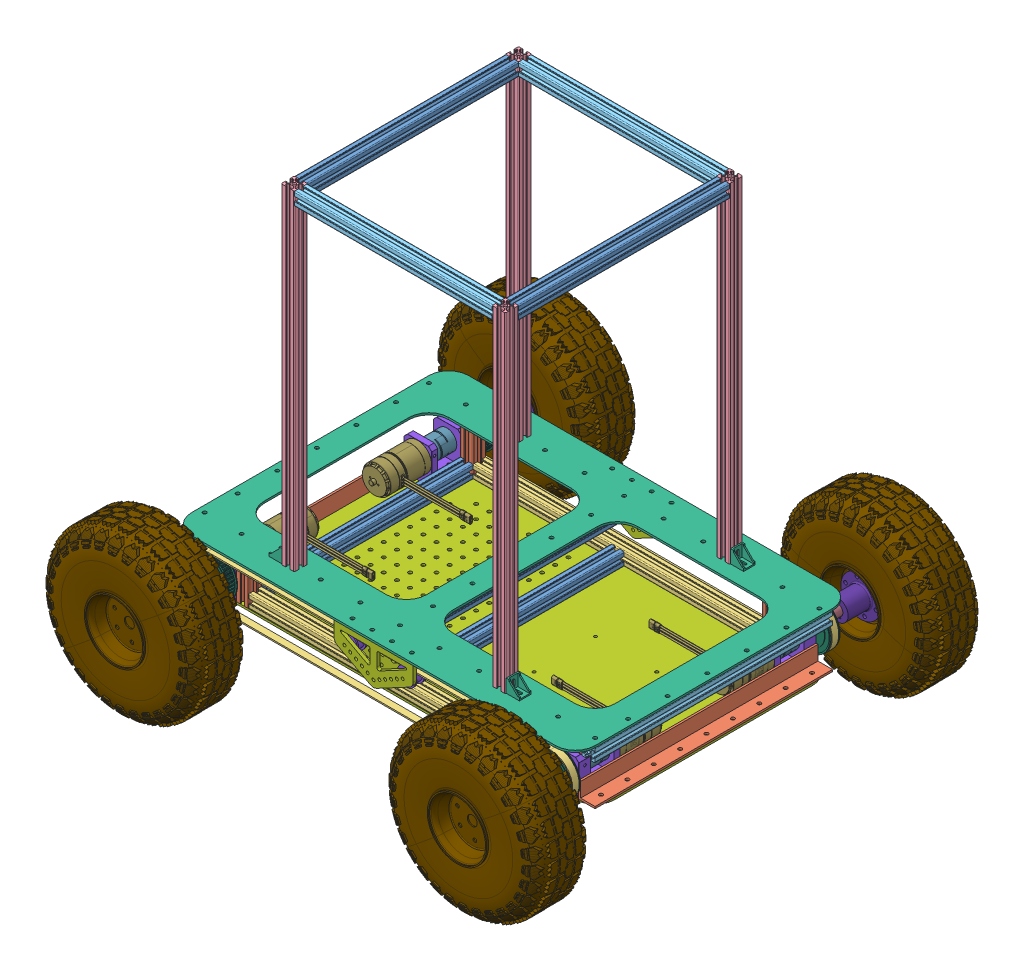
SolidWorks assembly 总装, configuration 默认. Lengths in mm.
Overall size (861.9 722.49 686.75).
130 component instances, 27 part files, 43 mates.
Components (placement in the parent):
- 框架-1: 框架 [默认] at (-91.5436 0.0792 612) size (612 80 360) (flexible)
  - 320-1: 320 [默认] at (-239 0 -160) size (20 20 320)
  - 60-1: 60 [默认] at (-239 0 160) x (0 0 1) z (0 1 0) size (20 20 60)
  - 60-2: 60 [默认] at (-239 60 -180) x (1 0 0) z (0 -1 0) size (20 20 60)
  - 438-1: 438 [默认] at (-219 0 180) x (0 0 -1) z (1 0 0) size (20 20 438)
  - 438-2: 438 [默认] at (-219 0 -160) x (0 0 -1) z (1 0 0) size (20 20 438)
  - 60-3: 60 [默认] at (219 60 -180) x (1 0 0) z (0 -1 0) size (20 20 60)
  - 60-4: 60 [默认] at (219 60 160) x (1 0 0) z (0 -1 0) size (20 20 60)
  - 320-2: 320 [默认] at (219 0 -160) size (20 20 320)
  - 572-3: 572 [默认] at (-286 60 180) x (0 0 -1) z (1 0 0) size (20 20 572)
  - 572-4: 572 [默认] at (-286 60 -160) x (0 0 -1) z (1 0 0) size (20 20 572)
  - 360-3: 360 [默认] at (-306 60 -180) size (20 20 360)
  - 360-4: 360 [默认] at (286 60 -180) size (20 20 360)
  - 320-3: 320 [默认] at (-10 60 -160) size (20 20 320)
  - 320-4: 320 [默认] at (-10 0 -160) size (20 20 320)
- 铝底板-上-1: 铝底板-上 [默认] at (-91.5436 80.0792 612) x (0 0 -1) z (1 0 0) size (420 3 612)
- 铝底板-下-1: 铝底板-下 [默认] at (-91.5436 -2.9208 612) x (0 0 1) z (-1 0 0) size (360 3 612)
- 轮胎模组-1: 轮胎模组 [默认] at (230.9564 22.3703 451.1678) x (0 0 -1) z (-1 0 0) size (297.23 295.63 295.43) (flexible)
  - m3508-1: m3508 [Default] at (-12.228 0.9134 62.5) size (62.5 52.5 42)
  - deep groove ball bearings gb-1: deep groove ball bearings gb [Rolling bearings 6000 GB 276-94] at (6.9178 -9.2089 62.5) size (8 26 26)
  - deep groove ball bearings gb-2: deep groove ball bearings gb [Rolling bearings 6000 GB 276-94] at (14.9178 -9.2089 62.5) x (1 0 0) z (0 0.136617 0.990624) size (8 26 26)
  - plain washers for clevis pins gb-1: plain washers for clevis pins gb [GB_ROUND_WASHERS_TYPE7 3] at (19.7178 1.5391 73.248) x (0 0 -1) z (1 0 0) size (6 6 0.8)
  - plain washers for clevis pins gb-2: plain washers for clevis pins gb [GB_ROUND_WASHERS_TYPE7 3] at (19.7178 1.5391 51.752) x (0 0 -1) z (1 0 0) size (6 6 0.8)
  - plain washers for clevis pins gb-3: plain washers for clevis pins gb [GB_ROUND_WASHERS_TYPE7 3] at (19.7178 -20.4006 72.7853) x (0 0 -1) z (1 0 0) size (6 6 0.8)
  - plain washers for clevis pins gb-4: plain washers for clevis pins gb [GB_ROUND_WASHERS_TYPE7 3] at (19.7178 -19.4942 51.3083) x (0 0 -1) z (1 0 0) size (6 6 0.8)
  - hexagon socket head cap screws gb-1: hexagon socket head cap screws gb [GB_FASTENER_SCREWS_HSHCS M3X8-N] at (22.7178 1.5391 73.248) x (-1 0 0) z (0 0.924225 0.381849) size (11 5.5 5.5)
  - hexagon socket head cap screws gb-2: hexagon socket head cap screws gb [GB_FASTENER_SCREWS_HSHCS M3X8-N] at (22.7178 1.5391 51.752) x (-1 0 0) z (0 0.924225 0.381849) size (11 5.5 5.5)
  - hexagon socket head cap screws gb-3: hexagon socket head cap screws gb [GB_FASTENER_SCREWS_HSHCS M3X8-N] at (22.7178 -20.4006 72.7853) x (-1 0 0) z (0 0.924225 0.381849) size (11 5.5 5.5)
  - hexagon socket head cap screws gb-4: hexagon socket head cap screws gb [GB_FASTENER_SCREWS_HSHCS M3X8-N] at (22.7178 -19.4942 51.3083) x (-1 0 0) z (0 0.924225 0.381849) size (11 5.5 5.5)
  - RoboMaster M3508直流无刷减速电-1: RoboMaster M3508直流无刷减速电 [默认] at (-130.0232 -5.4389 80.4643) x (0 -0.954008 0.299781) z (1 0 0) size (63.71 141.17 98.4)
  - 轴-1: 轴 [默认] at (18.9178 -9.2089 62.5) x (0 0.969975 -0.243205) z (0 0.243205 0.969975) size (16 128 16)
  - CPJCK30-RD-10-10-1: CPJCK30-RD-10-10 [Default] at (-34.3322 -9.2089 62.5) x (1 0 0) z (0 0.124503 0.992219) size (35 30 30)
  - 同步轮-1: 同步轮 [Default] at (28.0178 -9.2089 62.5) x (1 0 0) z (0 0.430878 0.90241) size (16 67 67)
  - 平键5x5x35-1: 平键5x5x35 [默认] at (94.4178 -1.9341 60.676) x (0 0.243205 0.969975) z (0 -0.969975 0.243205) size (5 41 5)
  - 法兰-1: 法兰 [默认] at (113.9178 -9.2089 62.5) x (0 -0.243205 -0.969975) z (1 0 0) size (60 60 41)
  - 10寸充气轮-1: 10寸充气轮 [Default] at (181.1138 -156.8863 150.0145) x (0 0.247823 -0.968805) z (1 0 0) size (242.76 243.05 91.75)
  - circlips for shaft--type a large gb-1: circlips for shaft--type a large gb [GB_CONNECTING_PIECE_RING_RRA 16] at (28.0178 -8.6289 62.5) x (0 0 -1) z (1 0 0) size (18.2 20.68 1)
  - circlips for shaft--type a large gb-2: circlips for shaft--type a large gb [GB_CONNECTING_PIECE_RING_RRA 16] at (44.0178 -8.6289 62.5) x (0 0 1) z (-1 0 0) size (18.2 20.68 1)
- 轮胎模组-2: 轮胎模组 [默认] at (105.9564 22.3703 772.8322) x (0 0 1) z (1 0 0) size (297.23 341.76 341.72) (flexible)
  - m3508-1: m3508 [Default] at (-12.228 0.9134 62.5) size (62.5 52.5 42)
  - deep groove ball bearings gb-1: deep groove ball bearings gb [Rolling bearings 6000 GB 276-94] at (6.9178 -9.2089 62.5) size (8 26 26)
  - deep groove ball bearings gb-2: deep groove ball bearings gb [Rolling bearings 6000 GB 276-94] at (14.9178 -9.2089 62.5) x (1 0 0) z (0 0.136617 0.990624) size (8 26 26)
  - plain washers for clevis pins gb-1: plain washers for clevis pins gb [GB_ROUND_WASHERS_TYPE7 3] at (19.7178 1.5391 73.248) x (0 0 -1) z (1 0 0) size (6 6 0.8)
  - plain washers for clevis pins gb-2: plain washers for clevis pins gb [GB_ROUND_WASHERS_TYPE7 3] at (19.7178 1.5391 51.752) x (0 0 -1) z (1 0 0) size (6 6 0.8)
  - plain washers for clevis pins gb-3: plain washers for clevis pins gb [GB_ROUND_WASHERS_TYPE7 3] at (19.7178 -20.4006 72.7853) x (0 0 -1) z (1 0 0) size (6 6 0.8)
  - plain washers for clevis pins gb-4: plain washers for clevis pins gb [GB_ROUND_WASHERS_TYPE7 3] at (19.7178 -19.4942 51.3083) x (0 0 -1) z (1 0 0) size (6 6 0.8)
  - hexagon socket head cap screws gb-1: hexagon socket head cap screws gb [GB_FASTENER_SCREWS_HSHCS M3X8-N] at (22.7178 1.5391 73.248) x (-1 0 0) z (0 0.924225 0.381849) size (11 5.5 5.5)
  - hexagon socket head cap screws gb-2: hexagon socket head cap screws gb [GB_FASTENER_SCREWS_HSHCS M3X8-N] at (22.7178 1.5391 51.752) x (-1 0 0) z (0 0.924225 0.381849) size (11 5.5 5.5)
  - hexagon socket head cap screws gb-3: hexagon socket head cap screws gb [GB_FASTENER_SCREWS_HSHCS M3X8-N] at (22.7178 -20.4006 72.7853) x (-1 0 0) z (0 0.924225 0.381849) size (11 5.5 5.5)
  - hexagon socket head cap screws gb-4: hexagon socket head cap screws gb [GB_FASTENER_SCREWS_HSHCS M3X8-N] at (22.7178 -19.4942 51.3083) x (-1 0 0) z (0 0.924225 0.381849) size (11 5.5 5.5)
  - RoboMaster M3508直流无刷减速电-1: RoboMaster M3508直流无刷减速电 [默认] at (-130.0232 -12.9789 44.5357) x (0 0.954008 -0.299781) z (1 0 0) size (63.71 141.17 98.4)
  - 轴-1: 轴 [默认] at (18.9178 -9.2089 62.5) x (0 0.982488 0.186325) z (0 -0.186325 0.982488) size (16 128 16)
  - CPJCK30-RD-10-10-1: CPJCK30-RD-10-10 [Default] at (-34.3322 -9.2089 62.5) x (1 0 0) z (0 0.124503 0.992219) size (35 30 30)
  - 同步轮-1: 同步轮 [Default] at (28.0178 -9.2089 62.5) size (16 67 67)
  - 平键5x5x35-1: 平键5x5x35 [默认] at (94.4178 -1.8402 63.8974) x (0 -0.186325 0.982488) z (0 -0.982488 -0.186325) size (5 41 5)
  - 法兰-1: 法兰 [默认] at (113.9178 -9.2089 62.5) x (0 0.186325 -0.982488) z (1 0 0) size (60 60 41)
  - 10寸充气轮-1: 10寸充气轮 [Default] at (181.1138 -179.9795 79.9579) x (0 0.631528 -0.775353) z (1 0 0) size (242.76 243.05 91.75)
  - circlips for shaft--type a large gb-1: circlips for shaft--type a large gb [GB_CONNECTING_PIECE_RING_RRA 16] at (28.0178 -8.6289 62.5) x (0 0 -1) z (1 0 0) size (18.2 20.68 1)
  - circlips for shaft--type a large gb-2: circlips for shaft--type a large gb [GB_CONNECTING_PIECE_RING_RRA 16] at (44.0178 -8.6289 62.5) x (0 0 1) z (-1 0 0) size (18.2 20.68 1)
- 轮胎模组-5: 轮胎模组 [默认] at (-289.0436 22.3703 451.1678) x (0 0 -1) z (-1 0 0) size (297.23 341.76 341.72) (flexible)
  - m3508-1: m3508 [Default] at (-12.228 0.9134 62.5) size (62.5 52.5 42)
  - deep groove ball bearings gb-1: deep groove ball bearings gb [Rolling bearings 6000 GB 276-94] at (6.9178 -9.2089 62.5) size (8 26 26)
  - deep groove ball bearings gb-2: deep groove ball bearings gb [Rolling bearings 6000 GB 276-94] at (14.9178 -9.2089 62.5) x (1 0 0) z (0 0.136617 0.990624) size (8 26 26)
  - plain washers for clevis pins gb-1: plain washers for clevis pins gb [GB_ROUND_WASHERS_TYPE7 3] at (19.7178 1.5391 73.248) x (0 0 -1) z (1 0 0) size (6 6 0.8)
  - plain washers for clevis pins gb-2: plain washers for clevis pins gb [GB_ROUND_WASHERS_TYPE7 3] at (19.7178 1.5391 51.752) x (0 0 -1) z (1 0 0) size (6 6 0.8)
  - plain washers for clevis pins gb-3: plain washers for clevis pins gb [GB_ROUND_WASHERS_TYPE7 3] at (19.7178 -20.4006 72.7853) x (0 0 -1) z (1 0 0) size (6 6 0.8)
  - plain washers for clevis pins gb-4: plain washers for clevis pins gb [GB_ROUND_WASHERS_TYPE7 3] at (19.7178 -19.4942 51.3083) x (0 0 -1) z (1 0 0) size (6 6 0.8)
  - hexagon socket head cap screws gb-1: hexagon socket head cap screws gb [GB_FASTENER_SCREWS_HSHCS M3X8-N] at (22.7178 1.5391 73.248) x (-1 0 0) z (0 0.924225 0.381849) size (11 5.5 5.5)
  - hexagon socket head cap screws gb-2: hexagon socket head cap screws gb [GB_FASTENER_SCREWS_HSHCS M3X8-N] at (22.7178 1.5391 51.752) x (-1 0 0) z (0 0.924225 0.381849) size (11 5.5 5.5)
  - hexagon socket head cap screws gb-3: hexagon socket head cap screws gb [GB_FASTENER_SCREWS_HSHCS M3X8-N] at (22.7178 -20.4006 72.7853) x (-1 0 0) z (0 0.924225 0.381849) size (11 5.5 5.5)
  - hexagon socket head cap screws gb-4: hexagon socket head cap screws gb [GB_FASTENER_SCREWS_HSHCS M3X8-N] at (22.7178 -19.4942 51.3083) x (-1 0 0) z (0 0.924225 0.381849) size (11 5.5 5.5)
  - RoboMaster M3508直流无刷减速电-1: RoboMaster M3508直流无刷减速电 [默认] at (-130.0232 -12.9789 44.5357) x (0 0.954008 -0.299781) z (1 0 0) size (63.71 141.17 98.4)
  - 轴-1: 轴 [默认] at (18.9178 -9.2089 62.5) x (0 0.982488 0.186325) z (0 -0.186325 0.982488) size (16 128 16)
  - CPJCK30-RD-10-10-1: CPJCK30-RD-10-10 [Default] at (-34.3322 -9.2089 62.5) x (1 0 0) z (0 0.124503 0.992219) size (35 30 30)
  - 同步轮-1: 同步轮 [Default] at (28.0178 -9.2089 62.5) size (16 67 67)
  - 平键5x5x35-1: 平键5x5x35 [默认] at (94.4178 -1.8402 63.8974) x (0 -0.186325 0.982488) z (0 -0.982488 -0.186325) size (5 41 5)
  - 法兰-1: 法兰 [默认] at (113.9178 -9.2089 62.5) x (0 0.186325 -0.982488) z (1 0 0) size (60 60 41)
  - 10寸充气轮-1: 10寸充气轮 [Default] at (181.1138 -179.9795 79.9579) x (0 0.631528 -0.775353) z (1 0 0) size (242.76 243.05 91.75)
  - circlips for shaft--type a large gb-1: circlips for shaft--type a large gb [GB_CONNECTING_PIECE_RING_RRA 16] at (28.0178 -8.6289 62.5) x (0 0 -1) z (1 0 0) size (18.2 20.68 1)
  - circlips for shaft--type a large gb-2: circlips for shaft--type a large gb [GB_CONNECTING_PIECE_RING_RRA 16] at (44.0178 -8.6289 62.5) x (0 0 1) z (-1 0 0) size (18.2 20.68 1)
- 轮胎模组-6: 轮胎模组 [默认] at (-414.0436 22.3703 772.8322) x (0 0 1) z (1 0 0) size (297.23 341.76 341.72) (flexible)
  - m3508-1: m3508 [Default] at (-12.228 0.9134 62.5) size (62.5 52.5 42)
  - deep groove ball bearings gb-1: deep groove ball bearings gb [Rolling bearings 6000 GB 276-94] at (6.9178 -9.2089 62.5) size (8 26 26)
  - deep groove ball bearings gb-2: deep groove ball bearings gb [Rolling bearings 6000 GB 276-94] at (14.9178 -9.2089 62.5) x (1 0 0) z (0 0.136617 0.990624) size (8 26 26)
  - plain washers for clevis pins gb-1: plain washers for clevis pins gb [GB_ROUND_WASHERS_TYPE7 3] at (19.7178 1.5391 73.248) x (0 0 -1) z (1 0 0) size (6 6 0.8)
  - plain washers for clevis pins gb-2: plain washers for clevis pins gb [GB_ROUND_WASHERS_TYPE7 3] at (19.7178 1.5391 51.752) x (0 0 -1) z (1 0 0) size (6 6 0.8)
  - plain washers for clevis pins gb-3: plain washers for clevis pins gb [GB_ROUND_WASHERS_TYPE7 3] at (19.7178 -20.4006 72.7853) x (0 0 -1) z (1 0 0) size (6 6 0.8)
  - plain washers for clevis pins gb-4: plain washers for clevis pins gb [GB_ROUND_WASHERS_TYPE7 3] at (19.7178 -19.4942 51.3083) x (0 0 -1) z (1 0 0) size (6 6 0.8)
  - hexagon socket head cap screws gb-1: hexagon socket head cap screws gb [GB_FASTENER_SCREWS_HSHCS M3X8-N] at (22.7178 1.5391 73.248) x (-1 0 0) z (0 0.924225 0.381849) size (11 5.5 5.5)
  - hexagon socket head cap screws gb-2: hexagon socket head cap screws gb [GB_FASTENER_SCREWS_HSHCS M3X8-N] at (22.7178 1.5391 51.752) x (-1 0 0) z (0 0.924225 0.381849) size (11 5.5 5.5)
  - hexagon socket head cap screws gb-3: hexagon socket head cap screws gb [GB_FASTENER_SCREWS_HSHCS M3X8-N] at (22.7178 -20.4006 72.7853) x (-1 0 0) z (0 0.924225 0.381849) size (11 5.5 5.5)
  - hexagon socket head cap screws gb-4: hexagon socket head cap screws gb [GB_FASTENER_SCREWS_HSHCS M3X8-N] at (22.7178 -19.4942 51.3083) x (-1 0 0) z (0 0.924225 0.381849) size (11 5.5 5.5)
  - RoboMaster M3508直流无刷减速电-1: RoboMaster M3508直流无刷减速电 [默认] at (-130.0232 -5.4389 80.4643) x (0 -0.954008 0.299781) z (1 0 0) size (63.71 141.17 98.4)
  - 轴-1: 轴 [默认] at (18.9178 -9.2089 62.5) x (0 0.982488 0.186325) z (0 -0.186325 0.982488) size (16 128 16)
  - CPJCK30-RD-10-10-1: CPJCK30-RD-10-10 [Default] at (-34.3322 -9.2089 62.5) x (1 0 0) z (0 0.124503 0.992219) size (35 30 30)
  - 同步轮-1: 同步轮 [Default] at (28.0178 -9.2089 62.5) size (16 67 67)
  - 平键5x5x35-1: 平键5x5x35 [默认] at (94.4178 -1.8402 63.8974) x (0 -0.186325 0.982488) z (0 -0.982488 -0.186325) size (5 41 5)
  - 法兰-1: 法兰 [默认] at (113.9178 -9.2089 62.5) x (0 0.186325 -0.982488) z (1 0 0) size (60 60 41)
  - 10寸充气轮-1: 10寸充气轮 [Default] at (181.1138 -179.9795 79.9579) x (0 0.631528 -0.775353) z (1 0 0) size (242.76 243.05 91.75)
  - circlips for shaft--type a large gb-1: circlips for shaft--type a large gb [GB_CONNECTING_PIECE_RING_RRA 16] at (28.0178 -8.6289 62.5) x (0 0 -1) z (1 0 0) size (18.2 20.68 1)
  - circlips for shaft--type a large gb-2: circlips for shaft--type a large gb [GB_CONNECTING_PIECE_RING_RRA 16] at (44.0178 -8.6289 62.5) x (0 0 1) z (-1 0 0) size (18.2 20.68 1)
- 直角铝-1: 直角铝 [默认] at (-375.5436 3.0792 612) x (0 0 -1) z (1 0 0) size (360 25 25)
- 直角铝-2: 直角铝 [默认] at (192.4564 3.0792 612) x (0 0 1) z (-1 0 0) size (360 25 25)
- 同步带-1: 同步带 [默认] at (168.4564 31.5792 813.85) x (0 0 -1) z (1 0 0) size (10 67.7 587.7)
- 同步带-2: 同步带 [默认] at (168.4564 31.5792 420.15) x (0 0 -1) z (1 0 0) size (10 67.7 587.7)
- 扩展架-1: 扩展架 [默认] at (62.0081 -166.9208 766.8893) x (0 0 -1) z (0 1 0) size (360 380 500)
  - 500-1: 500 [默认] at (-25.1107 -16.4483 250) size (20 20 500)
  - 500-2: 500 [默认] at (314.8893 -16.4483 250) size (20 20 500)
  - 500-3: 500 [默认] at (314.8893 303.5517 250) size (20 20 500)
  - 500-4: 500 [默认] at (-25.1107 303.5517 250) size (20 20 500)
  - 320-1: 320 [默认] at (-5.1107 3.5517 750) x (0 -1 0) z (1 0 0) size (20 20 320)
  - 320-2: 320 [默认] at (-5.1107 323.5517 730) x (0 0 1) z (1 0 0) size (20 20 320)
  - 300-1: 300 [默认] at (-25.1107 303.5517 730) x (1 0 0) z (0 -1 0) size (20 20 300)
  - 300-2: 300 [默认] at (314.8893 303.5517 730) x (1 0 0) z (0 -1 0) size (20 20 300)
  - 角码-1: 角码 [默认] at (995.5059 87.6877 1359.6334) x (0 -1 0) z (0 0 -1) size (20 17.5 20)
  - 角码-2: 角码 [默认] at (1335.5059 87.6877 1359.6334) x (0 -1 0) z (0 0 -1) size (20 17.5 20)
  - 角码-3: 角码 [默认] at (995.5059 -1126.0817 14.136) x (0 0 -1) z (0 1 0) size (20 17.5 20)
  - 角码-4: 角码 [默认] at (-685.7273 219.4156 1359.6334) x (0 1 0) z (0 0 -1) size (20 17.5 20)
- 张紧器-1: 张紧器 [默认] at (-91.5436 80.0792 808.85) x (0 0 1) z (-1 0 0) size (30.3 58.67 120)
  - 同步轮张紧器-1: 同步轮张紧器 [默认] at origin size (30.3 58.67 120)
  - 导向轮-1: 导向轮 [默认] at (0 -25.1373 -44.1176) size (15 28 28)
  - 钢柱4x15x8-1: 钢柱4x15x8 [默认] at (0 -25.1373 -44.1176) x (0 0 1) z (0 -1 0) size (8 16 8)
  - 导向轮-2: 导向轮 [默认] at (0 -25.1373 44.1176) x (1 0 0) z (0 -0.03847 0.99926) size (15 28 28)
  - 钢柱4x15x8-2: 钢柱4x15x8 [默认] at (0 -25.1373 44.1176) x (0 0 1) z (0 -1 0) size (8 16 8)
- 张紧器-2: 张紧器 [默认] at (-91.5436 80.0792 415.15) x (0 0 -1) z (1 0 0) size (30.3 58.67 120)
  - 同步轮张紧器-1: 同步轮张紧器 [默认] at origin size (30.3 58.67 120)
  - 导向轮-1: 导向轮 [默认] at (0 -25.1373 -44.1176) size (15 28 28)
  - 钢柱4x15x8-1: 钢柱4x15x8 [默认] at (0 -25.1373 -44.1176) x (0 0 1) z (0 -1 0) size (8 16 8)
  - 导向轮-2: 导向轮 [默认] at (0 -25.1373 44.1176) x (1 0 0) z (0 -0.03847 0.99926) size (15 28 28)
  - 钢柱4x15x8-2: 钢柱4x15x8 [默认] at (0 -25.1373 44.1176) x (0 0 1) z (0 -1 0) size (8 16 8)
Mates (geometry in assembly coordinates):
- Coincident1: coincident: plane of assembly; plane of assembly; plane of 框架-1/360-4 through (208.0564 80.0792 792) normal (0 1 0); plane of 铝底板-上-1 through (-91.5436 80.0792 612) normal (0 -1 0)
- Coincident3: coincident: plane of assembly; plane of assembly; plane of 框架-1/360-4 through (214.4564 73.6792 792) normal (1 0 0); plane of 铝底板-上-1 through (214.4564 83.0792 822) normal (1 0 0)
- Coincident4: coincident: plane of assembly; plane of assembly; plane of 框架-1/320-2 through (141.0564 0.0792 772) normal (0 -1 0); plane of 铝底板-下-1 through (-91.5436 0.0792 612) normal (0 1 0)
- Coincident5: coincident: plane of assembly; plane of assembly; plane of 铝底板-上-1 through (214.4564 83.0792 822) normal (1 0 0); plane of 铝底板-下-1 through (214.4564 0.0792 432) normal (1 0 0)
- Width1: width: plane of assembly; plane of assembly; plane of assembly; plane of assembly; plane of 铝底板-下-1 through (214.4564 0.0792 432) normal (0 0 -1); plane of 铝底板-下-1 through (214.4564 0.0792 792) normal (0 0 1); plane of 框架-1/438-1 through (127.4564 0.0792 792) normal (0 0 1); plane of 框架-1/438-2 through (127.4564 0.0792 432) normal (0 0 -1)
- Width2: width: plane of assembly; plane of assembly; plane of assembly; plane of assembly; plane of 铝底板-上-1 through (-397.5436 83.0792 822) normal (0 0 1); plane of 铝底板-上-1 through (-397.5436 83.0792 402) normal (0 0 -1); plane of 铝底板-下-1 through (214.4564 0.0792 432) normal (0 0 -1); plane of 铝底板-下-1 through (214.4564 0.0792 792) normal (0 0 1)
- Coincident6: coincident: plane of assembly; plane of assembly; plane of 铝底板-下-1 through (-91.5436 0.0792 612) normal (0 1 0); plane of 轮胎模组-1/m3508-1 through (147.4564 0.0792 494.75) normal (0 -1 0)
- Concentric1: concentric: cylinder of assembly; cylinder of assembly; cylinder of 铝底板-下-1 through (178.4564 0.0792 479) axis (0 -1 0) radius 2.75; cylinder of 轮胎模组-1/m3508-1 through (178.4564 7.0792 479) axis (0 -1 0) radius 2.55
- Concentric2: concentric: cylinder of assembly; cylinder of assembly; cylinder of 铝底板-下-1 through (178.4564 0.0792 457) axis (0 -1 0) radius 2.75; cylinder of 轮胎模组-1/m3508-1 through (178.4564 7.0792 457) axis (0 -1 0) radius 2.55
- Coincident7: coincident: plane of 铝底板-下-1 through (-91.5436 0.0792 612) normal (0 1 0); plane of 轮胎模组-2/m3508-1 through (189.4564 0.0792 729.25) normal (0 -1 0)
- Concentric3: concentric: cylinder of 铝底板-下-1 through (178.4564 0.0792 767) axis (0 -1 0) radius 2.75; cylinder of 轮胎模组-2/m3508-1 through (178.4564 7.0792 767) axis (0 -1 0) radius 2.55
- Concentric4: concentric: cylinder of 铝底板-下-1 through (178.4564 0.0792 745) axis (0 -1 0) radius 2.75; cylinder of 轮胎模组-2/m3508-1 through (178.4564 7.0792 745) axis (0 -1 0) radius 2.55
- Parallel1: parallel: plane of assembly; plane of assembly; plane of 框架-1/320-2 through (127.4564 0.0792 772) normal (-1 0 0); plane of 轮胎模组-2/RoboMaster M3508直流无刷减速电-1 through (44.6064 35.0792 685.9) normal (-1 0 0)
- Parallel2: parallel: plane of 框架-1/320-2 through (127.4564 0.0792 772) normal (-1 0 0); plane of 轮胎模组-1/RoboMaster M3508直流无刷减速电-1 through (44.6064 28.0792 538.1) normal (-1 0 0)
- Coincident8: coincident: plane of 铝底板-下-1 through (-91.5436 0.0792 612) normal (0 1 0); plane of 轮胎模组-5/m3508-1 through (-372.5436 0.0792 494.75) normal (0 -1 0)
- Coincident9: coincident: plane of 铝底板-下-1 through (-91.5436 0.0792 612) normal (0 1 0); plane of 轮胎模组-6/m3508-1 through (-330.5436 0.0792 729.25) normal (0 -1 0)
- Concentric5: concentric: cylinder of 铝底板-下-1 through (-361.5436 0.0792 745) axis (0 -1 0) radius 2.75; cylinder of 轮胎模组-6/m3508-1 through (-361.5436 7.0792 745) axis (0 -1 0) radius 2.55
- Concentric6: concentric: cylinder of 铝底板-下-1 through (-361.5436 0.0792 767) axis (0 -1 0) radius 2.75; cylinder of 轮胎模组-6/m3508-1 through (-361.5436 7.0792 767) axis (0 -1 0) radius 2.55
- Concentric7: concentric: cylinder of 铝底板-下-1 through (-361.5436 0.0792 457) axis (0 -1 0) radius 2.75; cylinder of 轮胎模组-5/m3508-1 through (-361.5436 7.0792 457) axis (0 -1 0) radius 2.55
- Concentric8: concentric: cylinder of 铝底板-下-1 through (-361.5436 0.0792 479) axis (0 -1 0) radius 2.75; cylinder of 轮胎模组-5/m3508-1 through (-361.5436 7.0792 479) axis (0 -1 0) radius 2.55
- Parallel3: parallel: plane of 框架-1/320-1 through (-310.5436 13.6792 772) normal (1 0 0); plane of 轮胎模组-5/RoboMaster M3508直流无刷减速电-1 through (-227.6936 35.0792 538.1) normal (1 0 0)
- Parallel4: parallel: plane of 框架-1/320-1 through (-310.5436 13.6792 772) normal (1 0 0); plane of 轮胎模组-6/RoboMaster M3508直流无刷减速电-1 through (-227.6936 28.0792 685.9) normal (1 0 0)
- Coincident10: coincident: plane of assembly; plane of assembly; plane of 铝底板-下-1 through (-91.5436 0.0792 612) normal (0 1 0); plane of 直角铝-1 through (-397.5436 0.0792 432) normal (0 -1 0)
- Concentric9: concentric: cylinder of assembly; cylinder of assembly; cylinder of 铝底板-下-1 through (-386.5436 -2.9208 452) axis (0 1 0) radius 2.75; cylinder of 直角铝-1 through (-386.5436 0.0792 452) axis (0 1 0) radius 2.75
- Concentric10: concentric: cylinder of assembly; cylinder of assembly; cylinder of 铝底板-下-1 through (-386.5436 -2.9208 492) axis (0 1 0) radius 2.75; cylinder of 直角铝-1 through (-386.5436 0.0792 492) axis (0 1 0) radius 2.75
- Coincident11: coincident: plane of assembly; plane of assembly; plane of 铝底板-下-1 through (-91.5436 0.0792 612) normal (0 1 0); plane of 直角铝-2 through (214.4564 0.0792 792) normal (0 -1 0)
- Concentric11: concentric: cylinder of assembly; cylinder of assembly; cylinder of 铝底板-下-1 through (203.4564 -2.9208 772) axis (0 1 0) radius 2.75; cylinder of 直角铝-2 through (203.4564 0.0792 772) axis (0 1 0) radius 2.75
- Concentric12: concentric: cylinder of assembly; cylinder of assembly; cylinder of 铝底板-下-1 through (203.4564 -2.9208 732) axis (0 1 0) radius 2.75; cylinder of 直角铝-2 through (203.4564 0.0792 732) axis (0 1 0) radius 2.75
- Concentric13: concentric: cylinder of assembly; cylinder of assembly; cylinder of 轮胎模组-2/轴-1 through (168.4564 31.5792 886.75) axis (0 0 -1) radius 8; cylinder of 同步带-1 through (168.4564 31.5792 803.85) axis (0 0 1) radius 31.85
- Concentric14: concentric: cylinder of 轮胎模组-6/轴-1 through (-351.5436 31.5792 886.75) axis (0 0 -1) radius 8; cylinder of 同步带-1 through (-351.5436 31.5792 803.85) axis (0 0 1) radius 31.85
- Width3: width: plane of assembly; plane of assembly; plane of assembly; plane of assembly; plane of 轮胎模组-6/同步轮-1 through (-351.5436 31.5792 800.85) normal (0 0 -1); plane of 轮胎模组-6/同步轮-1 through (-351.5436 6.5792 816.85) normal (0 0 1); plane of 同步带-1 through (168.4564 31.5792 813.85) normal (0 0 1); plane of 同步带-1 through (168.4564 31.5792 803.85) normal (0 0 -1)
- Concentric15: concentric: cylinder of 轮胎模组-5/轴-1 through (-351.5436 31.5792 337.25) axis (0 0 1) radius 8; cylinder of 同步带-2 through (-351.5436 31.5792 410.15) axis (0 0 1) radius 31.85
- Concentric16: concentric: cylinder of 轮胎模组-1/轴-1 through (168.4564 31.5792 337.25) axis (0 0 1) radius 8; cylinder of 同步带-2 through (168.4564 31.5792 410.15) axis (0 0 1) radius 31.85
- Width4: width: plane of 轮胎模组-1/同步轮-1 through (168.4564 31.5792 423.15) normal (0 0 1); plane of 轮胎模组-1/同步轮-1 through (179.2284 9.0189 407.15) normal (0 0 -1); plane of 同步带-2 through (168.4564 31.5792 410.15) normal (0 0 -1); plane of 同步带-2 through (168.4564 31.5792 420.15) normal (0 0 1)
- Coincident12: coincident: plane of assembly; plane of assembly; plane of 铝底板-上-1 through (-91.5436 83.0792 612) normal (0 1 0); plane of 扩展架-1/500-1 through (78.1564 83.0792 785.2) normal (0 -1 0)
- Width5: width: plane of assembly; plane of assembly; plane of assembly; plane of assembly; plane of 铝底板-上-1 through (-397.5436 83.0792 402) normal (0 0 -1); plane of 铝底板-上-1 through (-397.5436 83.0792 822) normal (0 0 1); plane of 扩展架-1/500-4 through (-255.1436 583.0792 792) normal (0 0 1); plane of 扩展架-1/500-3 through (-255.1436 583.0792 432) normal (0 0 -1)
- Width6: width: plane of assembly; plane of assembly; plane of assembly; plane of assembly; plane of 铝底板-上-1 through (-397.5436 83.0792 822) normal (-1 0 0); plane of 铝底板-上-1 through (214.4564 83.0792 822) normal (1 0 0); plane of 扩展架-1/500-2 through (78.4564 583.0792 438.4) normal (1 0 0); plane of 扩展架-1/500-3 through (-261.5436 583.0792 438.4) normal (-1 0 0)
- Concentric17: concentric: cylinder of assembly; cylinder of assembly; cylinder of 铝底板-上-1 through (-46.5436 80.0792 808.85) axis (0 1 0) radius 2.75; cylinder of 张紧器-1/同步轮张紧器-1 through (-46.5436 20.0792 808.85) axis (0 1 0) radius 2.75
- Concentric18: concentric: cylinder of assembly; cylinder of assembly; cylinder of 铝底板-上-1 through (-136.5436 80.0792 808.85) axis (0 1 0) radius 2.75; cylinder of 张紧器-1/同步轮张紧器-1 through (-136.5436 20.0792 808.85) axis (0 1 0) radius 2.75
- Coincident13: coincident: plane of assembly; plane of assembly; plane of 铝底板-上-1 through (-91.5436 80.0792 612) normal (0 -1 0); plane of 张紧器-1/同步轮张紧器-1 through (-151.5436 80.0792 822) normal (0 1 0)
- Coincident14: coincident: plane of assembly; plane of assembly; plane of 铝底板-上-1 through (-91.5436 80.0792 612) normal (0 -1 0); plane of 张紧器-2/同步轮张紧器-1 through (-31.5436 80.0792 402) normal (0 1 0)
- Concentric19: concentric: cylinder of assembly; cylinder of assembly; cylinder of 铝底板-上-1 through (-136.5436 80.0792 415.15) axis (0 1 0) radius 2.75; cylinder of 张紧器-2/同步轮张紧器-1 through (-136.5436 20.0792 415.15) axis (0 1 0) radius 2.75
- Concentric20: concentric: cylinder of assembly; cylinder of assembly; cylinder of 铝底板-上-1 through (-46.5436 80.0792 415.15) axis (0 1 0) radius 2.75; cylinder of 张紧器-2/同步轮张紧器-1 through (-46.5436 20.0792 415.15) axis (0 1 0) radius 2.75
